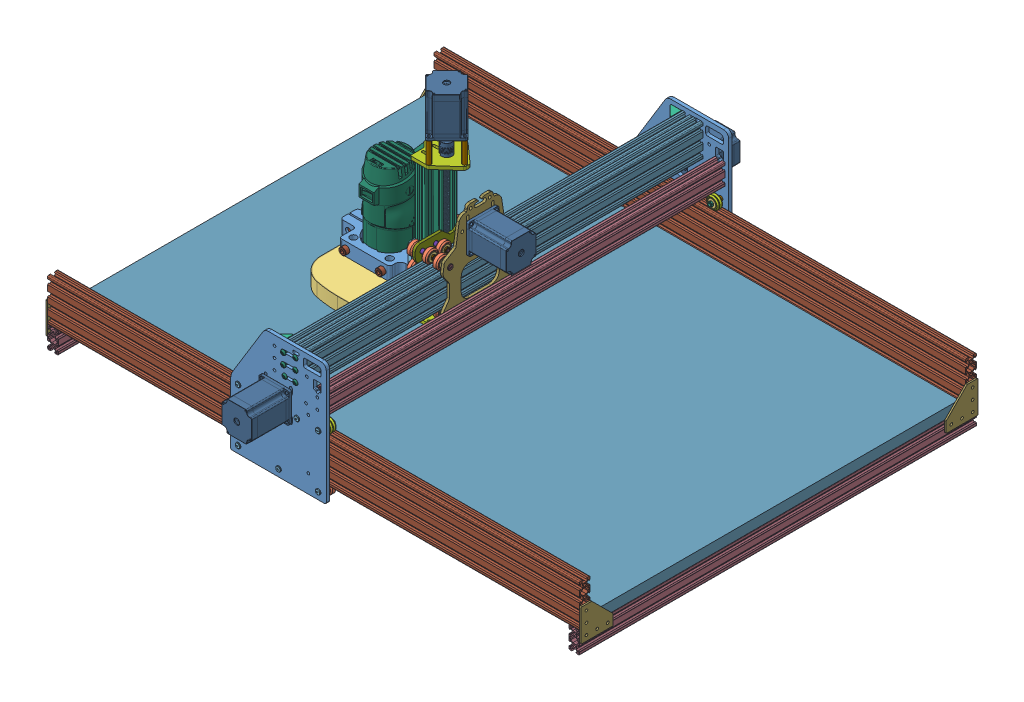
SolidWorks assembly MainFrame, configuration Default. Lengths in mm.
Overall size (1006.09 487.54 917.5).
449 component instances, 49 part files, 68 mates.
Components (placement in the parent):
- LeftSideGantry-1: LeftSideGantry [Default] at (4.6712 -16.6579 18.9022) size (180.04 227.49 106.2)
  - Gantry-SidePlate-1: Gantry-SidePlate [Default] at (69.6077 16.1075 4.3758) size (180.04 227.49 6.35)
  - SolidWheelWithEccentric-1: SolidWheelWithEccentric [Default] at (93.8735 -103.2758 -22.2954) size (23.89 23.89 29.6)
    - Delrin Solid V-Wheel-1: Delrin Solid V-Wheel [Default] at (-54.4571 19.9667 15.1712) size (23.89 23.89 10.23)
    - Precision Ball Bearing-1: Precision Ball Bearing [Default] at (-54.4571 19.9667 12.1712) x (0 0 1) z (-1 0 0) size (5 16 16)
    - Precision Ball Bearing-2: Precision Ball Bearing [Default] at (-54.4571 19.9667 18.1712) x (0 0 -1) z (1 0 0) size (5 16 16)
    - Steel Eccentric Spacer-1: Steel Eccentric Spacer [Default] at (-55.2471 19.9667 26.6712) x (0 0 -1) z (1 0 0) size (7.27 9.09 7.9)
    - 5mm Low Profile Socket Head Screw - Multiple Lengths-1: 5mm Low Profile Socket Head Screw - Multiple Lengths [Default] at (-54.4571 19.9667 34.7712) x (0 0 -1) z (1 0 0) size (27.2 9.5 9.5)
    - Nylon Insert Hex Locknut 5mm-1: Nylon Insert Hex Locknut 5mm [Default] at (-54.4571 19.9667 9.6712) x (-0.923728 -0.383049 0) z (0 0 -1) size (7.68 8.82 4.5)
  - SolidWheelWithEccentric-2: SolidWheelWithEccentric [Default] at (19.3435 -103.2758 -22.2954) size (23.89 23.89 29.6)
    - Delrin Solid V-Wheel-1: Delrin Solid V-Wheel [Default] at (-54.4571 19.9667 15.1712) size (23.89 23.89 10.23)
    - Precision Ball Bearing-1: Precision Ball Bearing [Default] at (-54.4571 19.9667 12.1712) x (0 0 1) z (-1 0 0) size (5 16 16)
    - Precision Ball Bearing-2: Precision Ball Bearing [Default] at (-54.4571 19.9667 18.1712) x (0 0 -1) z (1 0 0) size (5 16 16)
    - Steel Eccentric Spacer-1: Steel Eccentric Spacer [Default] at (-55.2471 19.9667 26.6712) x (0 0 -1) z (1 0 0) size (7.27 9.09 7.9)
    - 5mm Low Profile Socket Head Screw - Multiple Lengths-1: 5mm Low Profile Socket Head Screw - Multiple Lengths [Default] at (-54.4571 19.9667 34.7712) x (0 0 -1) z (1 0 0) size (27.2 9.5 9.5)
    - Nylon Insert Hex Locknut 5mm-1: Nylon Insert Hex Locknut 5mm [Default] at (-54.4571 19.9667 9.6712) x (-0.923728 -0.383049 0) z (0 0 -1) size (7.68 8.82 4.5)
  - SolidWheelWithEccentric-3: SolidWheelWithEccentric [Default] at (-56.7665 -103.2758 -22.2954) size (23.89 23.89 29.6)
    - Delrin Solid V-Wheel-1: Delrin Solid V-Wheel [Default] at (-54.4571 19.9667 15.1712) size (23.89 23.89 10.23)
    - Precision Ball Bearing-1: Precision Ball Bearing [Default] at (-54.4571 19.9667 12.1712) x (0 0 1) z (-1 0 0) size (5 16 16)
    - Precision Ball Bearing-2: Precision Ball Bearing [Default] at (-54.4571 19.9667 18.1712) x (0 0 -1) z (1 0 0) size (5 16 16)
    - Steel Eccentric Spacer-1: Steel Eccentric Spacer [Default] at (-55.2471 19.9667 26.6712) x (0 0 -1) z (1 0 0) size (7.27 9.09 7.9)
    - 5mm Low Profile Socket Head Screw - Multiple Lengths-1: 5mm Low Profile Socket Head Screw - Multiple Lengths [Default] at (-54.4571 19.9667 34.7712) x (0 0 -1) z (1 0 0) size (27.2 9.5 9.5)
    - Nylon Insert Hex Locknut 5mm-1: Nylon Insert Hex Locknut 5mm [Default] at (-54.4571 19.9667 9.6712) x (-0.923728 -0.383049 0) z (0 0 -1) size (7.68 8.82 4.5)
  - V-Slot Delrin Dual Wheel Assembly-1: V-Slot Delrin Dual Wheel Assembly [Default] at (-115.4002 2.9807 3.6104) size (23.89 23.89 29.95)
    - Delrin Dual V-Wheel-1: Delrin Dual V-Wheel [Default] at (4.1766 13.0717 -11.0846) size (23.89 23.89 10.23)
    - Precision Ball Bearing-1: Precision Ball Bearing [Default] at (4.1766 13.0717 -8.0846) x (0 0 -1) z (1 0 0) size (5 16 16)
    - Precision Ball Bearing-2: Precision Ball Bearing [Default] at (4.1766 13.0717 -14.0846) x (0 0 -1) z (1 0 0) size (5 16 16)
    - 5mm Precision Washer-1: 5mm Precision Washer [Default] at (4.1766 13.0717 -11.5846) x (0 0 1) z (-1 0 0) size (1 10 10)
    - .25 Inch Aluminum Spacer-1: .25 Inch Aluminum Spacer [Default] at (4.1766 13.0717 0.7654) x (0 0 -1) z (1 0 0) size (6.35 8 8)
    - 5mm Low Profile Socket Head Screw - Multiple Lengths-1: 5mm Low Profile Socket Head Screw - Multiple Lengths [Default] at (4.1766 13.0717 8.8654) x (0 0 -1) z (1 0 0) size (27.2 9.5 9.5)
    - Nylon Insert Hex Locknut 5mm-1: Nylon Insert Hex Locknut 5mm [Default] at (4.1766 13.0717 -16.5846) x (-0.923728 -0.383049 0) z (0 0 -1) size (7.68 8.82 4.5)
  - V-Slot Delrin Dual Wheel Assembly-2: V-Slot Delrin Dual Wheel Assembly [Default] at (-75.4002 2.9807 3.6104) size (23.89 23.89 29.95)
    - Delrin Dual V-Wheel-1: Delrin Dual V-Wheel [Default] at (4.1766 13.0717 -11.0846) size (23.89 23.89 10.23)
    - Precision Ball Bearing-1: Precision Ball Bearing [Default] at (4.1766 13.0717 -8.0846) x (0 0 -1) z (1 0 0) size (5 16 16)
    - Precision Ball Bearing-2: Precision Ball Bearing [Default] at (4.1766 13.0717 -14.0846) x (0 0 -1) z (1 0 0) size (5 16 16)
    - 5mm Precision Washer-1: 5mm Precision Washer [Default] at (4.1766 13.0717 -11.5846) x (0 0 1) z (-1 0 0) size (1 10 10)
    - .25 Inch Aluminum Spacer-1: .25 Inch Aluminum Spacer [Default] at (4.1766 13.0717 0.7654) x (0 0 -1) z (1 0 0) size (6.35 8 8)
    - 5mm Low Profile Socket Head Screw - Multiple Lengths-1: 5mm Low Profile Socket Head Screw - Multiple Lengths [Default] at (4.1766 13.0717 8.8654) x (0 0 -1) z (1 0 0) size (27.2 9.5 9.5)
    - Nylon Insert Hex Locknut 5mm-1: Nylon Insert Hex Locknut 5mm [Default] at (4.1766 13.0717 -16.5846) x (-0.923728 -0.383049 0) z (0 0 -1) size (7.68 8.82 4.5)
  - V-Slot Delrin Dual Wheel Assembly-3: V-Slot Delrin Dual Wheel Assembly [Default] at (35.1946 3.1996 3.6104) size (23.89 23.89 29.95)
    - Delrin Dual V-Wheel-1: Delrin Dual V-Wheel [Default] at (4.1766 13.0717 -11.0846) size (23.89 23.89 10.23)
    - Precision Ball Bearing-1: Precision Ball Bearing [Default] at (4.1766 13.0717 -8.0846) x (0 0 -1) z (1 0 0) size (5 16 16)
    - Precision Ball Bearing-2: Precision Ball Bearing [Default] at (4.1766 13.0717 -14.0846) x (0 0 -1) z (1 0 0) size (5 16 16)
    - 5mm Precision Washer-1: 5mm Precision Washer [Default] at (4.1766 13.0717 -11.5846) x (0 0 1) z (-1 0 0) size (1 10 10)
    - .25 Inch Aluminum Spacer-1: .25 Inch Aluminum Spacer [Default] at (4.1766 13.0717 0.7654) x (0 0 -1) z (1 0 0) size (6.35 8 8)
    - 5mm Low Profile Socket Head Screw - Multiple Lengths-1: 5mm Low Profile Socket Head Screw - Multiple Lengths [Default] at (4.1766 13.0717 8.8654) x (0 0 -1) z (1 0 0) size (27.2 9.5 9.5)
    - Nylon Insert Hex Locknut 5mm-1: Nylon Insert Hex Locknut 5mm [Default] at (4.1766 13.0717 -16.5846) x (-0.923728 -0.383049 0) z (0 0 -1) size (7.68 8.82 4.5)
  - V-Slot Delrin Dual Wheel Assembly-4: V-Slot Delrin Dual Wheel Assembly [Default] at (-4.7602 2.9807 3.6104) size (23.89 23.89 29.95)
    - Delrin Dual V-Wheel-1: Delrin Dual V-Wheel [Default] at (4.1766 13.0717 -11.0846) size (23.89 23.89 10.23)
    - Precision Ball Bearing-1: Precision Ball Bearing [Default] at (4.1766 13.0717 -8.0846) x (0 0 -1) z (1 0 0) size (5 16 16)
    - Precision Ball Bearing-2: Precision Ball Bearing [Default] at (4.1766 13.0717 -14.0846) x (0 0 -1) z (1 0 0) size (5 16 16)
    - 5mm Precision Washer-1: 5mm Precision Washer [Default] at (4.1766 13.0717 -11.5846) x (0 0 1) z (-1 0 0) size (1 10 10)
    - .25 Inch Aluminum Spacer-1: .25 Inch Aluminum Spacer [Default] at (4.1766 13.0717 0.7654) x (0 0 -1) z (1 0 0) size (6.35 8 8)
    - 5mm Low Profile Socket Head Screw - Multiple Lengths-1: 5mm Low Profile Socket Head Screw - Multiple Lengths [Default] at (4.1766 13.0717 8.8654) x (0 0 -1) z (1 0 0) size (27.2 9.5 9.5)
    - Nylon Insert Hex Locknut 5mm-1: Nylon Insert Hex Locknut 5mm [Default] at (4.1766 13.0717 -16.5846) x (-0.923728 -0.383049 0) z (0 0 -1) size (7.68 8.82 4.5)
  - stepper motor NEMA 23 57x76-1: stepper motor NEMA 23 57x76 [По умолчанию] at (-36.1116 31.8353 88.7258) x (0.999999 0.00168 0) z (-0.00168 0.999999 0) size (56.67 96.5 56.58)
- vslot_20_x_80-1: vslot_20_x_80 [Default] at (526.5598 -49.8299 11.278) x (0.001454 -0.999999 0) z (-0.999999 -0.001454 0) size (80 20 1000)
- RightSideGantry-1: RightSideGantry [Default] at (45.1481 -36.7387 -745.9581) size (182.59 229.13 105)
  - Gantry-SidePlate-1: Gantry-SidePlate [Default] at (29.1308 36.1882 12.8861) size (180.04 227.49 6.35)
  - V-Slot Delrin Dual Wheel Assembly-1: V-Slot Delrin Dual Wheel Assembly [Default] at (-120.5656 46.608 20.0014) x (0.923728 0.383049 0) z (0 0 -1) size (23.89 23.89 29.95)
    - Delrin Dual V-Wheel-1: Delrin Dual V-Wheel [Default] at (4.1766 13.0717 -11.0846) size (23.89 23.89 10.23)
    - Precision Ball Bearing-1: Precision Ball Bearing [Default] at (4.1766 13.0717 -8.0846) x (0 0 -1) z (1 0 0) size (5 16 16)
    - Precision Ball Bearing-2: Precision Ball Bearing [Default] at (4.1766 13.0717 -14.0846) x (0 0 -1) z (1 0 0) size (5 16 16)
    - 5mm Precision Washer-1: 5mm Precision Washer [Default] at (4.1766 13.0717 -11.5846) x (0 0 1) z (-1 0 0) size (1 10 10)
    - .25 Inch Aluminum Spacer-1: .25 Inch Aluminum Spacer [Default] at (4.1766 13.0717 0.7654) x (0 0 -1) z (1 0 0) size (6.35 8 8)
    - 5mm Low Profile Socket Head Screw - Multiple Lengths-1: 5mm Low Profile Socket Head Screw - Multiple Lengths [Default] at (4.1766 13.0717 8.8654) x (0 0 -1) z (1 0 0) size (27.2 9.5 9.5)
    - Nylon Insert Hex Locknut 5mm-1: Nylon Insert Hex Locknut 5mm [Default] at (4.1766 13.0717 -16.5846) x (-0.923728 -0.383049 0) z (0 0 -1) size (7.68 8.82 4.5)
  - V-Slot Delrin Dual Wheel Assembly-2: V-Slot Delrin Dual Wheel Assembly [Default] at (-160.5656 46.608 20.0014) x (0.923728 0.383049 0) z (0 0 -1) size (23.89 23.89 29.95)
    - Delrin Dual V-Wheel-1: Delrin Dual V-Wheel [Default] at (4.1766 13.0717 -11.0846) size (23.89 23.89 10.23)
    - Precision Ball Bearing-1: Precision Ball Bearing [Default] at (4.1766 13.0717 -8.0846) x (0 0 -1) z (1 0 0) size (5 16 16)
    - Precision Ball Bearing-2: Precision Ball Bearing [Default] at (4.1766 13.0717 -14.0846) x (0 0 -1) z (1 0 0) size (5 16 16)
    - 5mm Precision Washer-1: 5mm Precision Washer [Default] at (4.1766 13.0717 -11.5846) x (0 0 1) z (-1 0 0) size (1 10 10)
    - .25 Inch Aluminum Spacer-1: .25 Inch Aluminum Spacer [Default] at (4.1766 13.0717 0.7654) x (0 0 -1) z (1 0 0) size (6.35 8 8)
    - 5mm Low Profile Socket Head Screw - Multiple Lengths-1: 5mm Low Profile Socket Head Screw - Multiple Lengths [Default] at (4.1766 13.0717 8.8654) x (0 0 -1) z (1 0 0) size (27.2 9.5 9.5)
    - Nylon Insert Hex Locknut 5mm-1: Nylon Insert Hex Locknut 5mm [Default] at (4.1766 13.0717 -16.5846) x (-0.923728 -0.383049 0) z (0 0 -1) size (7.68 8.82 4.5)
  - V-Slot Delrin Dual Wheel Assembly-3: V-Slot Delrin Dual Wheel Assembly [Default] at (7.7594 25.8772 20.0014) x (-0.923728 -0.383049 0) z (0 0 -1) size (23.89 23.89 29.95)
    - Delrin Dual V-Wheel-1: Delrin Dual V-Wheel [Default] at (4.1766 13.0717 -11.0846) size (23.89 23.89 10.23)
    - Precision Ball Bearing-1: Precision Ball Bearing [Default] at (4.1766 13.0717 -8.0846) x (0 0 -1) z (1 0 0) size (5 16 16)
    - Precision Ball Bearing-2: Precision Ball Bearing [Default] at (4.1766 13.0717 -14.0846) x (0 0 -1) z (1 0 0) size (5 16 16)
    - 5mm Precision Washer-1: 5mm Precision Washer [Default] at (4.1766 13.0717 -11.5846) x (0 0 1) z (-1 0 0) size (1 10 10)
    - .25 Inch Aluminum Spacer-1: .25 Inch Aluminum Spacer [Default] at (4.1766 13.0717 0.7654) x (0 0 -1) z (1 0 0) size (6.35 8 8)
    - 5mm Low Profile Socket Head Screw - Multiple Lengths-1: 5mm Low Profile Socket Head Screw - Multiple Lengths [Default] at (4.1766 13.0717 8.8654) x (0 0 -1) z (1 0 0) size (27.2 9.5 9.5)
    - Nylon Insert Hex Locknut 5mm-1: Nylon Insert Hex Locknut 5mm [Default] at (4.1766 13.0717 -16.5846) x (-0.923728 -0.383049 0) z (0 0 -1) size (7.68 8.82 4.5)
  - V-Slot Delrin Dual Wheel Assembly-4: V-Slot Delrin Dual Wheel Assembly [Default] at (-32.1954 25.6582 20.0014) x (-0.923728 -0.383049 0) z (0 0 -1) size (23.89 23.89 29.95)
    - Delrin Dual V-Wheel-1: Delrin Dual V-Wheel [Default] at (4.1766 13.0717 -11.0846) size (23.89 23.89 10.23)
    - Precision Ball Bearing-1: Precision Ball Bearing [Default] at (4.1766 13.0717 -8.0846) x (0 0 -1) z (1 0 0) size (5 16 16)
    - Precision Ball Bearing-2: Precision Ball Bearing [Default] at (4.1766 13.0717 -14.0846) x (0 0 -1) z (1 0 0) size (5 16 16)
    - 5mm Precision Washer-1: 5mm Precision Washer [Default] at (4.1766 13.0717 -11.5846) x (0 0 1) z (-1 0 0) size (1 10 10)
    - .25 Inch Aluminum Spacer-1: .25 Inch Aluminum Spacer [Default] at (4.1766 13.0717 0.7654) x (0 0 -1) z (1 0 0) size (6.35 8 8)
    - 5mm Low Profile Socket Head Screw - Multiple Lengths-1: 5mm Low Profile Socket Head Screw - Multiple Lengths [Default] at (4.1766 13.0717 8.8654) x (0 0 -1) z (1 0 0) size (27.2 9.5 9.5)
    - Nylon Insert Hex Locknut 5mm-1: Nylon Insert Hex Locknut 5mm [Default] at (4.1766 13.0717 -16.5846) x (-0.923728 -0.383049 0) z (0 0 -1) size (7.68 8.82 4.5)
  - SolidWheelWithEccentric-1: SolidWheelWithEccentric [Default] at (-108.3154 -23.6223 45.9073) x (0.923728 0.383049 0) z (0 0 -1) size (23.89 23.89 29.6)
    - Delrin Solid V-Wheel-1: Delrin Solid V-Wheel [Default] at (-54.4571 19.9667 15.1712) size (23.89 23.89 10.23)
    - Precision Ball Bearing-1: Precision Ball Bearing [Default] at (-54.4571 19.9667 12.1712) x (0 0 1) z (-1 0 0) size (5 16 16)
    - Precision Ball Bearing-2: Precision Ball Bearing [Default] at (-54.4571 19.9667 18.1712) x (0 0 -1) z (1 0 0) size (5 16 16)
    - Steel Eccentric Spacer-1: Steel Eccentric Spacer [Default] at (-55.2471 19.9667 26.6712) x (0 0 -1) z (1 0 0) size (7.27 9.09 7.9)
    - 5mm Low Profile Socket Head Screw - Multiple Lengths-1: 5mm Low Profile Socket Head Screw - Multiple Lengths [Default] at (-54.4571 19.9667 34.7712) x (0 0 -1) z (1 0 0) size (27.2 9.5 9.5)
    - Nylon Insert Hex Locknut 5mm-1: Nylon Insert Hex Locknut 5mm [Default] at (-54.4571 19.9667 9.6712) x (-0.923728 -0.383049 0) z (0 0 -1) size (7.68 8.82 4.5)
  - SolidWheelWithEccentric-2: SolidWheelWithEccentric [Default] at (-32.9954 -23.6223 45.9073) x (0.923728 0.383049 0) z (0 0 -1) size (23.89 23.89 29.6)
    - Delrin Solid V-Wheel-1: Delrin Solid V-Wheel [Default] at (-54.4571 19.9667 15.1712) size (23.89 23.89 10.23)
    - Precision Ball Bearing-1: Precision Ball Bearing [Default] at (-54.4571 19.9667 12.1712) x (0 0 1) z (-1 0 0) size (5 16 16)
    - Precision Ball Bearing-2: Precision Ball Bearing [Default] at (-54.4571 19.9667 18.1712) x (0 0 -1) z (1 0 0) size (5 16 16)
    - Steel Eccentric Spacer-1: Steel Eccentric Spacer [Default] at (-55.2471 19.9667 26.6712) x (0 0 -1) z (1 0 0) size (7.27 9.09 7.9)
    - 5mm Low Profile Socket Head Screw - Multiple Lengths-1: 5mm Low Profile Socket Head Screw - Multiple Lengths [Default] at (-54.4571 19.9667 34.7712) x (0 0 -1) z (1 0 0) size (27.2 9.5 9.5)
    - Nylon Insert Hex Locknut 5mm-1: Nylon Insert Hex Locknut 5mm [Default] at (-54.4571 19.9667 9.6712) x (-0.923728 -0.383049 0) z (0 0 -1) size (7.68 8.82 4.5)
  - SolidWheelWithEccentric-3: SolidWheelWithEccentric [Default] at (42.3246 -23.6223 45.9073) x (0.923728 0.383049 0) z (0 0 -1) size (23.89 23.89 29.6)
    - Delrin Solid V-Wheel-1: Delrin Solid V-Wheel [Default] at (-54.4571 19.9667 15.1712) size (23.89 23.89 10.23)
    - Precision Ball Bearing-1: Precision Ball Bearing [Default] at (-54.4571 19.9667 12.1712) x (0 0 1) z (-1 0 0) size (5 16 16)
    - Precision Ball Bearing-2: Precision Ball Bearing [Default] at (-54.4571 19.9667 18.1712) x (0 0 -1) z (1 0 0) size (5 16 16)
    - Steel Eccentric Spacer-1: Steel Eccentric Spacer [Default] at (-55.2471 19.9667 26.6712) x (0 0 -1) z (1 0 0) size (7.27 9.09 7.9)
    - 5mm Low Profile Socket Head Screw - Multiple Lengths-1: 5mm Low Profile Socket Head Screw - Multiple Lengths [Default] at (-54.4571 19.9667 34.7712) x (0 0 -1) z (1 0 0) size (27.2 9.5 9.5)
    - Nylon Insert Hex Locknut 5mm-1: Nylon Insert Hex Locknut 5mm [Default] at (-54.4571 19.9667 9.6712) x (-0.923728 -0.383049 0) z (0 0 -1) size (7.68 8.82 4.5)
  - stepper motor NEMA 23 57x76-1: stepper motor NEMA 23 57x76 [По умолчанию] at (-76.1724 47.1139 -63.9139) x (1 0 0) z (0 -1 0) size (56.67 96.5 56.58)
- vslot_20_x_80-2: vslot_20_x_80 [Default] at (526.5598 -49.8299 -714.722) x (0.001454 -0.999999 0) z (-0.999999 -0.001454 0) size (80 20 1000)
- CrossSlideAssembly-1: CrossSlideAssembly [Default] at (27.0126 95.3807 -262.4793) x (0 0 1) z (-1 0 0) size (140.04 177.38 107.28)
  - Gantry-Mount-1: Gantry-Mount [Default] at (-125.7398 -49.8559 3.7822) size (140.04 177.38 9.53)
  - Steel Eccentric Spacer-1: Steel Eccentric Spacer [Default] at (-94.6645 20.3573 14.5772) x (0 0 1) z (-0.00681 0.999977 0) size (7.27 9.09 7.9)
  - Steel Eccentric Spacer-2: Steel Eccentric Spacer [Default] at (19.1018 20.3573 14.5772) x (0 0 1) z (-0.00681 0.999977 0) size (7.27 9.09 7.9)
  - .25 Inch Aluminum Spacer-3: .25 Inch Aluminum Spacer [Default] at (19.1049 -57.7227 19.6572) x (0 0 -1) z (1 0 0) size (6.35 8 8)
  - .25 Inch Aluminum Spacer-4: .25 Inch Aluminum Spacer [Default] at (-94.6784 -57.7227 19.6572) x (0 0 -1) z (1 0 0) size (6.35 8 8)
  - SolidWheel-7: SolidWheel [Default] at (56.5607 -62.4006 9.4904) size (23.89 23.89 11)
    - Delrin Solid V-Wheel-1: Delrin Solid V-Wheel [Default] at (-37.4558 4.6779 16.5868) size (23.89 23.89 10.23)
    - Precision Ball Bearing-1: Precision Ball Bearing [Default] at (-37.4558 4.6779 19.5868) x (0 0 -1) z (1 0 0) size (5 16 16)
    - Precision Ball Bearing-2: Precision Ball Bearing [Default] at (-37.4558 4.6779 13.5868) x (0 0 1) z (-1 0 0) size (5 16 16)
  - SolidWheel-8: SolidWheel [Default] at (56.5522 16.4694 9.4904) size (23.89 23.89 11)
    - Delrin Solid V-Wheel-1: Delrin Solid V-Wheel [Default] at (-37.4558 4.6779 16.5868) size (23.89 23.89 10.23)
    - Precision Ball Bearing-1: Precision Ball Bearing [Default] at (-37.4558 4.6779 19.5868) x (0 0 -1) z (1 0 0) size (5 16 16)
    - Precision Ball Bearing-2: Precision Ball Bearing [Default] at (-37.4558 4.6779 13.5868) x (0 0 1) z (-1 0 0) size (5 16 16)
  - SolidWheel-9: SolidWheel [Default] at (-57.2141 16.4694 9.4904) size (23.89 23.89 11)
    - Delrin Solid V-Wheel-1: Delrin Solid V-Wheel [Default] at (-37.4558 4.6779 16.5868) size (23.89 23.89 10.23)
    - Precision Ball Bearing-1: Precision Ball Bearing [Default] at (-37.4558 4.6779 19.5868) x (0 0 -1) z (1 0 0) size (5 16 16)
    - Precision Ball Bearing-2: Precision Ball Bearing [Default] at (-37.4558 4.6779 13.5868) x (0 0 1) z (-1 0 0) size (5 16 16)
  - SolidWheel-10: SolidWheel [Default] at (-57.2226 -62.4006 9.4904) size (23.89 23.89 11)
    - Delrin Solid V-Wheel-1: Delrin Solid V-Wheel [Default] at (-37.4558 4.6779 16.5868) size (23.89 23.89 10.23)
    - Precision Ball Bearing-1: Precision Ball Bearing [Default] at (-37.4558 4.6779 19.5868) x (0 0 -1) z (1 0 0) size (5 16 16)
    - Precision Ball Bearing-2: Precision Ball Bearing [Default] at (-37.4558 4.6779 13.5868) x (0 0 1) z (-1 0 0) size (5 16 16)
  - Low Profile Socket Head Screw-2: Low Profile Socket Head Screw [Default] at (19.0964 21.1473 6.7947) x (0 0 1) z (-0.923728 -0.383049 0) size (32.23 9.5 9.5)
  - Low Profile Socket Head Screw-3: Low Profile Socket Head Screw [Default] at (-94.6699 21.1473 6.7947) x (0 0 1) z (-0.923728 -0.383049 0) size (32.23 9.5 9.5)
  - Low Profile Socket Head Screw-11: Low Profile Socket Head Screw [Default] at (19.1049 -57.7227 6.7947) x (0 0 1) z (-0.923728 -0.383049 0) size (32.23 9.5 9.5)
  - Low Profile Socket Head Screw-12: Low Profile Socket Head Screw [Default] at (-94.6784 -57.7227 6.7947) x (0 0 1) z (-0.923728 -0.383049 0) size (32.23 9.5 9.5)
  - stepper motor NEMA 23 57x76-1: stepper motor NEMA 23 57x76 [По умолчанию] at (-37.9748 53.7319 -68.2553) x (1 0 0) z (0 -1 0) size (56.67 96.5 56.58)
- vslot 20 x 60-1: vslot 20 x 60 [Default] at (6.4261 6.4154 -443.5992) x (0 -1 0) z (0 0 -1) size (60 20 770.25)
  - vslot_20_x_60-1: vslot_20_x_60 [Default] at (-59.9677 5.5907 273.1228) size (60 20 750)
  - socket button head cap screw_am-1: socket button head cap screw_am [B18.3.4M - 5 x 0.8 x 16 SBHCS --N] at (-49.9677 5.5907 291.8728) x (0 0 -1) z (1 0 0) size (18.75 9.5 9.5)
  - socket button head cap screw_am-2: socket button head cap screw_am [B18.3.4M - 5 x 0.8 x 16 SBHCS --N] at (-69.9677 5.5907 294.6228) x (0 0 -1) z (1 0 0) size (18.75 9.5 9.5)
  - socket button head cap screw_am-3: socket button head cap screw_am [B18.3.4M - 5 x 0.8 x 16 SBHCS --N] at (-89.9677 5.5907 294.6228) x (0 0 -1) z (1 0 0) size (18.75 9.5 9.5)
  - socket button head cap screw_am-4: socket button head cap screw_am [B18.3.4M - 5 x 0.8 x 16 SBHCS --N] at (-89.9677 5.5907 -475.6272) x (0 0 1) z (-1 0 0) size (18.75 9.5 9.5)
  - socket button head cap screw_am-5: socket button head cap screw_am [B18.3.4M - 5 x 0.8 x 16 SBHCS --N] at (-69.9677 5.5907 -475.6272) x (0 0 1) z (-1 0 0) size (18.75 9.5 9.5)
  - socket button head cap screw_am-6: socket button head cap screw_am [B18.3.4M - 5 x 0.8 x 16 SBHCS --N] at (-49.9677 5.5907 -475.6272) x (0 0 1) z (0.888663 -0.45856 0) size (18.75 9.5 9.5)
- vslot 20 x 60-2: vslot 20 x 60 [Default] at (-24.7553 6.4154 -259.8448) x (0 -1 0) z (0 0 1) size (60 20 770.25)
  - vslot_20_x_60-1: vslot_20_x_60 [Default] at (-59.9677 5.5907 273.1228) size (60 20 750)
  - socket button head cap screw_am-1: socket button head cap screw_am [B18.3.4M - 5 x 0.8 x 16 SBHCS --N] at (-49.9677 5.5907 291.8728) x (0 0 -1) z (1 0 0) size (18.75 9.5 9.5)
  - socket button head cap screw_am-2: socket button head cap screw_am [B18.3.4M - 5 x 0.8 x 16 SBHCS --N] at (-69.9677 5.5907 294.6228) x (0 0 -1) z (1 0 0) size (18.75 9.5 9.5)
  - socket button head cap screw_am-3: socket button head cap screw_am [B18.3.4M - 5 x 0.8 x 16 SBHCS --N] at (-89.9677 5.5907 294.6228) x (0 0 -1) z (1 0 0) size (18.75 9.5 9.5)
  - socket button head cap screw_am-4: socket button head cap screw_am [B18.3.4M - 5 x 0.8 x 16 SBHCS --N] at (-89.9677 5.5907 -475.6272) x (0 0 1) z (-1 0 0) size (18.75 9.5 9.5)
  - socket button head cap screw_am-5: socket button head cap screw_am [B18.3.4M - 5 x 0.8 x 16 SBHCS --N] at (-69.9677 5.5907 -475.6272) x (0 0 1) z (-1 0 0) size (18.75 9.5 9.5)
  - socket button head cap screw_am-6: socket button head cap screw_am [B18.3.4M - 5 x 0.8 x 16 SBHCS --N] at (-49.9677 5.5907 -475.6272) x (0 0 1) z (0.888663 -0.45856 0) size (18.75 9.5 9.5)
- FrontGantryPlateZaxis-1: FrontGantryPlateZaxis [Default] at (-15.5555 68.0354 -249.6907) x (0 0 1) z (-1 0 0) size (140.04 377.73 80.67)
  - Gantry-Mount-Part2-1: Gantry-Mount-Part2 [Default] at (-50.6115 110.7452 18.3591) size (140.04 106.72 4.76)
  - SolidWheelWithSpacer-4: SolidWheelWithSpacer [Default] at (-86.321 51.345 -9.6249) size (23.89 23.89 32.23)
    - SolidWheel-1: SolidWheel [Default] at (16.2383 -7.5303 -3.4528) size (23.89 23.89 11)
      - Delrin Solid V-Wheel-1: Delrin Solid V-Wheel [Default] at (-37.4558 4.6779 16.5868) size (23.89 23.89 10.23)
      - Precision Ball Bearing-1: Precision Ball Bearing [Default] at (-37.4558 4.6779 19.5868) x (0 0 -1) z (1 0 0) size (5 16 16)
      - Precision Ball Bearing-2: Precision Ball Bearing [Default] at (-37.4558 4.6779 13.5868) x (0 0 1) z (-1 0 0) size (5 16 16)
    - Low Profile Socket Head Screw-1: Low Profile Socket Head Screw [Default] at (-21.2174 -2.8524 35.734) x (0 0 -1) z (-0.923728 -0.383049 0) size (32.23 9.5 9.5)
    - .25 Inch Nylon Spacer-1: .25 Inch Nylon Spacer [Default] at (-21.2174 -2.8524 27.984) x (0 0 -1) z (1 0 0) size (6.35 7.94 7.94)
    - hex nut jam_am-1: hex nut jam_am [B18.2.4.5M - Hex jam nut,  M5 x 0.8 --D-N] at (-21.2174 -2.8524 7.634) size (8 9.24 2.7)
    - 3mm Aluminum Spacer-1: 3mm Aluminum Spacer [Default] at (-21.2174 -2.8524 21.634) x (0 0 -1) z (1 0 0) size (3 8 8)
  - SolidWheelWithSpacer-5: SolidWheelWithSpacer [Default] at (27.5253 51.345 -9.6249) size (23.89 23.89 32.23)
    - SolidWheel-1: SolidWheel [Default] at (16.2383 -7.5303 -3.4528) size (23.89 23.89 11)
      - Delrin Solid V-Wheel-1: Delrin Solid V-Wheel [Default] at (-37.4558 4.6779 16.5868) size (23.89 23.89 10.23)
      - Precision Ball Bearing-1: Precision Ball Bearing [Default] at (-37.4558 4.6779 19.5868) x (0 0 -1) z (1 0 0) size (5 16 16)
      - Precision Ball Bearing-2: Precision Ball Bearing [Default] at (-37.4558 4.6779 13.5868) x (0 0 1) z (-1 0 0) size (5 16 16)
    - Low Profile Socket Head Screw-1: Low Profile Socket Head Screw [Default] at (-21.2174 -2.8524 35.734) x (0 0 -1) z (-0.923728 -0.383049 0) size (32.23 9.5 9.5)
    - .25 Inch Nylon Spacer-1: .25 Inch Nylon Spacer [Default] at (-21.2174 -2.8524 27.984) x (0 0 -1) z (1 0 0) size (6.35 7.94 7.94)
    - hex nut jam_am-1: hex nut jam_am [B18.2.4.5M - Hex jam nut,  M5 x 0.8 --D-N] at (-21.2174 -2.8524 7.634) size (8 9.24 2.7)
    - 3mm Aluminum Spacer-1: 3mm Aluminum Spacer [Default] at (-21.2174 -2.8524 21.634) x (0 0 -1) z (1 0 0) size (3 8 8)
  - SolidWheelWithEccentric2-4: SolidWheelWithEccentric2 [Default] at (-75.4106 -21.8202 -18.8913) size (23.89 23.89 32.23)
    - SolidWheel-1: SolidWheel [Default] at (5.3595 -13.235 6.1636) size (23.89 23.89 11)
      - Delrin Solid V-Wheel-1: Delrin Solid V-Wheel [Default] at (-37.4558 4.6779 16.5868) size (23.89 23.89 10.23)
      - Precision Ball Bearing-1: Precision Ball Bearing [Default] at (-37.4558 4.6779 19.5868) x (0 0 -1) z (1 0 0) size (5 16 16)
      - Precision Ball Bearing-2: Precision Ball Bearing [Default] at (-37.4558 4.6779 13.5868) x (0 0 1) z (-1 0 0) size (5 16 16)
    - Steel Eccentric Spacer-1: Steel Eccentric Spacer [Default] at (-32.1017 -9.3471 37.2504) x (0 0 -1) z (0.00681 0.999977 0) size (7.27 9.09 7.9)
    - Low Profile Socket Head Screw-1: Low Profile Socket Head Screw [Default] at (-32.0963 -8.5571 45.0004) x (0 0 -1) z (1 0 0) size (32.23 9.5 9.5)
    - hex nut jam_am-1: hex nut jam_am [B18.2.4.5M - Hex jam nut,  M5 x 0.8 --D-N] at (-32.0963 -8.5571 17.2504) size (8 9.24 2.7)
    - 3mm Aluminum Spacer-1: 3mm Aluminum Spacer [Default] at (-32.0963 -8.5571 31.2504) x (0 0 -1) z (1 0 0) size (3 8 8)
  - SolidWheelWithEccentric2-5: SolidWheelWithEccentric2 [Default] at (38.3727 -21.8202 -18.8913) size (23.89 23.89 32.23)
    - SolidWheel-1: SolidWheel [Default] at (5.3595 -13.235 6.1636) size (23.89 23.89 11)
      - Delrin Solid V-Wheel-1: Delrin Solid V-Wheel [Default] at (-37.4558 4.6779 16.5868) size (23.89 23.89 10.23)
      - Precision Ball Bearing-1: Precision Ball Bearing [Default] at (-37.4558 4.6779 19.5868) x (0 0 -1) z (1 0 0) size (5 16 16)
      - Precision Ball Bearing-2: Precision Ball Bearing [Default] at (-37.4558 4.6779 13.5868) x (0 0 1) z (-1 0 0) size (5 16 16)
    - Steel Eccentric Spacer-1: Steel Eccentric Spacer [Default] at (-32.1017 -9.3471 37.2504) x (0 0 -1) z (0.00681 0.999977 0) size (7.27 9.09 7.9)
    - Low Profile Socket Head Screw-1: Low Profile Socket Head Screw [Default] at (-32.0963 -8.5571 45.0004) x (0 0 -1) z (1 0 0) size (32.23 9.5 9.5)
    - hex nut jam_am-1: hex nut jam_am [B18.2.4.5M - Hex jam nut,  M5 x 0.8 --D-N] at (-32.0963 -8.5571 17.2504) size (8 9.24 2.7)
    - 3mm Aluminum Spacer-1: 3mm Aluminum Spacer [Default] at (-32.0963 -8.5571 31.2504) x (0 0 -1) z (1 0 0) size (3 8 8)
  - SolidWheelWithSpacer-6: SolidWheelWithSpacer [Default] at (-61.321 51.345 -9.6249) size (23.89 23.89 32.23)
    - SolidWheel-1: SolidWheel [Default] at (16.2383 -7.5303 -3.4528) size (23.89 23.89 11)
      - Delrin Solid V-Wheel-1: Delrin Solid V-Wheel [Default] at (-37.4558 4.6779 16.5868) size (23.89 23.89 10.23)
      - Precision Ball Bearing-1: Precision Ball Bearing [Default] at (-37.4558 4.6779 19.5868) x (0 0 -1) z (1 0 0) size (5 16 16)
      - Precision Ball Bearing-2: Precision Ball Bearing [Default] at (-37.4558 4.6779 13.5868) x (0 0 1) z (-1 0 0) size (5 16 16)
    - Low Profile Socket Head Screw-1: Low Profile Socket Head Screw [Default] at (-21.2174 -2.8524 35.734) x (0 0 -1) z (-0.923728 -0.383049 0) size (32.23 9.5 9.5)
    - .25 Inch Nylon Spacer-1: .25 Inch Nylon Spacer [Default] at (-21.2174 -2.8524 27.984) x (0 0 -1) z (1 0 0) size (6.35 7.94 7.94)
    - hex nut jam_am-1: hex nut jam_am [B18.2.4.5M - Hex jam nut,  M5 x 0.8 --D-N] at (-21.2174 -2.8524 7.634) size (8 9.24 2.7)
    - 3mm Aluminum Spacer-1: 3mm Aluminum Spacer [Default] at (-21.2174 -2.8524 21.634) x (0 0 -1) z (1 0 0) size (3 8 8)
  - SolidWheelWithSpacer-7: SolidWheelWithSpacer [Default] at (2.5253 51.345 -9.6249) size (23.89 23.89 32.23)
    - SolidWheel-1: SolidWheel [Default] at (16.2383 -7.5303 -3.4528) size (23.89 23.89 11)
      - Delrin Solid V-Wheel-1: Delrin Solid V-Wheel [Default] at (-37.4558 4.6779 16.5868) size (23.89 23.89 10.23)
      - Precision Ball Bearing-1: Precision Ball Bearing [Default] at (-37.4558 4.6779 19.5868) x (0 0 -1) z (1 0 0) size (5 16 16)
      - Precision Ball Bearing-2: Precision Ball Bearing [Default] at (-37.4558 4.6779 13.5868) x (0 0 1) z (-1 0 0) size (5 16 16)
    - Low Profile Socket Head Screw-1: Low Profile Socket Head Screw [Default] at (-21.2174 -2.8524 35.734) x (0 0 -1) z (-0.923728 -0.383049 0) size (32.23 9.5 9.5)
    - .25 Inch Nylon Spacer-1: .25 Inch Nylon Spacer [Default] at (-21.2174 -2.8524 27.984) x (0 0 -1) z (1 0 0) size (6.35 7.94 7.94)
    - hex nut jam_am-1: hex nut jam_am [B18.2.4.5M - Hex jam nut,  M5 x 0.8 --D-N] at (-21.2174 -2.8524 7.634) size (8 9.24 2.7)
    - 3mm Aluminum Spacer-1: 3mm Aluminum Spacer [Default] at (-21.2174 -2.8524 21.634) x (0 0 -1) z (1 0 0) size (3 8 8)
  - V-Slot Spacer Block-1: V-Slot Spacer Block [Default] at (-90.5311 -1.2477 29.1216) x (0.000018 -1 0) z (0 0 -1) size (86 20 12)
  - V-Slot_Spacer_Block_Eccentric-1: V-Slot_Spacer_Block_Eccentric [Default] at (-10.8992 -1.2477 29.1216) x (-0.000396 1 0) z (0 0 1) size (86 20 12)
  - 8mm Acme Nut Block-1: 8mm Acme Nut Block [Default] at (-50.5861 18.7523 29.1216) x (1 0 0) z (0 1 0) size (34 12 20.51)
  - SolidWheelWithEccentric2-6: SolidWheelWithEccentric2 [Default] at (18.5024 13.3172 72.372) x (0.975301 -0.220879 0) z (0 0 -1) size (23.89 23.89 32.23)
    - SolidWheel-1: SolidWheel [Default] at (5.3595 -13.235 6.1636) size (23.89 23.89 11)
      - Delrin Solid V-Wheel-1: Delrin Solid V-Wheel [Default] at (-37.4558 4.6779 16.5868) size (23.89 23.89 10.23)
      - Precision Ball Bearing-1: Precision Ball Bearing [Default] at (-37.4558 4.6779 19.5868) x (0 0 -1) z (1 0 0) size (5 16 16)
      - Precision Ball Bearing-2: Precision Ball Bearing [Default] at (-37.4558 4.6779 13.5868) x (0 0 1) z (-1 0 0) size (5 16 16)
    - Steel Eccentric Spacer-1: Steel Eccentric Spacer [Default] at (-32.1017 -9.3471 37.2504) x (0 0 -1) z (0.00681 0.999977 0) size (7.27 9.09 7.9)
    - Low Profile Socket Head Screw-1: Low Profile Socket Head Screw [Default] at (-32.0963 -8.5571 45.0004) x (0 0 -1) z (1 0 0) size (32.23 9.5 9.5)
    - hex nut jam_am-1: hex nut jam_am [B18.2.4.5M - Hex jam nut,  M5 x 0.8 --D-N] at (-32.0963 -8.5571 17.2504) size (8 9.24 2.7)
    - 3mm Aluminum Spacer-1: 3mm Aluminum Spacer [Default] at (-32.0963 -8.5571 31.2504) x (0 0 -1) z (1 0 0) size (3 8 8)
  - SolidWheelWithEccentric2-7: SolidWheelWithEccentric2 [Default] at (-43.8134 -35.6376 72.372) x (-0.923728 -0.383049 0) z (0 0 -1) size (23.89 23.89 32.23)
    - SolidWheel-1: SolidWheel [Default] at (5.3595 -13.235 6.1636) size (23.89 23.89 11)
      - Delrin Solid V-Wheel-1: Delrin Solid V-Wheel [Default] at (-37.4558 4.6779 16.5868) size (23.89 23.89 10.23)
      - Precision Ball Bearing-1: Precision Ball Bearing [Default] at (-37.4558 4.6779 19.5868) x (0 0 -1) z (1 0 0) size (5 16 16)
      - Precision Ball Bearing-2: Precision Ball Bearing [Default] at (-37.4558 4.6779 13.5868) x (0 0 1) z (-1 0 0) size (5 16 16)
    - Steel Eccentric Spacer-1: Steel Eccentric Spacer [Default] at (-32.1017 -9.3471 37.2504) x (0 0 -1) z (0.00681 0.999977 0) size (7.27 9.09 7.9)
    - Low Profile Socket Head Screw-1: Low Profile Socket Head Screw [Default] at (-32.0963 -8.5571 45.0004) x (0 0 -1) z (1 0 0) size (32.23 9.5 9.5)
    - hex nut jam_am-1: hex nut jam_am [B18.2.4.5M - Hex jam nut,  M5 x 0.8 --D-N] at (-32.0963 -8.5571 17.2504) size (8 9.24 2.7)
    - 3mm Aluminum Spacer-1: 3mm Aluminum Spacer [Default] at (-32.0963 -8.5571 31.2504) x (0 0 -1) z (1 0 0) size (3 8 8)
  - SolidWheelWithEccentric2-8: SolidWheelWithEccentric2 [Default] at (-43.8253 -5.6376 72.372) x (-0.923728 -0.383049 0) z (0 0 -1) size (23.89 23.89 32.23)
    - SolidWheel-1: SolidWheel [Default] at (5.3595 -13.235 6.1636) size (23.89 23.89 11)
      - Delrin Solid V-Wheel-1: Delrin Solid V-Wheel [Default] at (-37.4558 4.6779 16.5868) size (23.89 23.89 10.23)
      - Precision Ball Bearing-1: Precision Ball Bearing [Default] at (-37.4558 4.6779 19.5868) x (0 0 -1) z (1 0 0) size (5 16 16)
      - Precision Ball Bearing-2: Precision Ball Bearing [Default] at (-37.4558 4.6779 13.5868) x (0 0 1) z (-1 0 0) size (5 16 16)
    - Steel Eccentric Spacer-1: Steel Eccentric Spacer [Default] at (-32.1017 -9.3471 37.2504) x (0 0 -1) z (0.00681 0.999977 0) size (7.27 9.09 7.9)
    - Low Profile Socket Head Screw-1: Low Profile Socket Head Screw [Default] at (-32.0963 -8.5571 45.0004) x (0 0 -1) z (1 0 0) size (32.23 9.5 9.5)
    - hex nut jam_am-1: hex nut jam_am [B18.2.4.5M - Hex jam nut,  M5 x 0.8 --D-N] at (-32.0963 -8.5571 17.2504) size (8 9.24 2.7)
    - 3mm Aluminum Spacer-1: 3mm Aluminum Spacer [Default] at (-32.0963 -8.5571 31.2504) x (0 0 -1) z (1 0 0) size (3 8 8)
  - SolidWheelWithSpacer-8: SolidWheelWithSpacer [Default] at (-111.2233 23.2598 63.1056) x (-0.923728 -0.383049 0) z (0 0 -1) size (23.89 23.89 32.23)
    - SolidWheel-1: SolidWheel [Default] at (16.2383 -7.5303 -3.4528) size (23.89 23.89 11)
      - Delrin Solid V-Wheel-1: Delrin Solid V-Wheel [Default] at (-37.4558 4.6779 16.5868) size (23.89 23.89 10.23)
      - Precision Ball Bearing-1: Precision Ball Bearing [Default] at (-37.4558 4.6779 19.5868) x (0 0 -1) z (1 0 0) size (5 16 16)
      - Precision Ball Bearing-2: Precision Ball Bearing [Default] at (-37.4558 4.6779 13.5868) x (0 0 1) z (-1 0 0) size (5 16 16)
    - Low Profile Socket Head Screw-1: Low Profile Socket Head Screw [Default] at (-21.2174 -2.8524 35.734) x (0 0 -1) z (-0.923728 -0.383049 0) size (32.23 9.5 9.5)
    - .25 Inch Nylon Spacer-1: .25 Inch Nylon Spacer [Default] at (-21.2174 -2.8524 27.984) x (0 0 -1) z (1 0 0) size (6.35 7.94 7.94)
    - hex nut jam_am-1: hex nut jam_am [B18.2.4.5M - Hex jam nut,  M5 x 0.8 --D-N] at (-21.2174 -2.8524 7.634) size (8 9.24 2.7)
    - 3mm Aluminum Spacer-1: 3mm Aluminum Spacer [Default] at (-21.2174 -2.8524 21.634) x (0 0 -1) z (1 0 0) size (3 8 8)
  - SolidWheelWithSpacer-9: SolidWheelWithSpacer [Default] at (-69.8393 4.2448 63.1056) x (0.923728 0.383049 0) z (0 0 -1) size (23.89 23.89 32.23)
    - SolidWheel-1: SolidWheel [Default] at (16.2383 -7.5303 -3.4528) size (23.89 23.89 11)
      - Delrin Solid V-Wheel-1: Delrin Solid V-Wheel [Default] at (-37.4558 4.6779 16.5868) size (23.89 23.89 10.23)
      - Precision Ball Bearing-1: Precision Ball Bearing [Default] at (-37.4558 4.6779 19.5868) x (0 0 -1) z (1 0 0) size (5 16 16)
      - Precision Ball Bearing-2: Precision Ball Bearing [Default] at (-37.4558 4.6779 13.5868) x (0 0 1) z (-1 0 0) size (5 16 16)
    - Low Profile Socket Head Screw-1: Low Profile Socket Head Screw [Default] at (-21.2174 -2.8524 35.734) x (0 0 -1) z (-0.923728 -0.383049 0) size (32.23 9.5 9.5)
    - .25 Inch Nylon Spacer-1: .25 Inch Nylon Spacer [Default] at (-21.2174 -2.8524 27.984) x (0 0 -1) z (1 0 0) size (6.35 7.94 7.94)
    - hex nut jam_am-1: hex nut jam_am [B18.2.4.5M - Hex jam nut,  M5 x 0.8 --D-N] at (-21.2174 -2.8524 7.634) size (8 9.24 2.7)
    - 3mm Aluminum Spacer-1: 3mm Aluminum Spacer [Default] at (-21.2174 -2.8524 21.634) x (0 0 -1) z (1 0 0) size (3 8 8)
  - SolidWheelWithSpacer-10: SolidWheelWithSpacer [Default] at (-111.2223 -36.7402 63.1056) x (-0.923728 -0.383049 0) z (0 0 -1) size (23.89 23.89 32.23)
    - SolidWheel-1: SolidWheel [Default] at (16.2383 -7.5303 -3.4528) size (23.89 23.89 11)
      - Delrin Solid V-Wheel-1: Delrin Solid V-Wheel [Default] at (-37.4558 4.6779 16.5868) size (23.89 23.89 10.23)
      - Precision Ball Bearing-1: Precision Ball Bearing [Default] at (-37.4558 4.6779 19.5868) x (0 0 -1) z (1 0 0) size (5 16 16)
      - Precision Ball Bearing-2: Precision Ball Bearing [Default] at (-37.4558 4.6779 13.5868) x (0 0 1) z (-1 0 0) size (5 16 16)
    - Low Profile Socket Head Screw-1: Low Profile Socket Head Screw [Default] at (-21.2174 -2.8524 35.734) x (0 0 -1) z (-0.923728 -0.383049 0) size (32.23 9.5 9.5)
    - .25 Inch Nylon Spacer-1: .25 Inch Nylon Spacer [Default] at (-21.2174 -2.8524 27.984) x (0 0 -1) z (1 0 0) size (6.35 7.94 7.94)
    - hex nut jam_am-1: hex nut jam_am [B18.2.4.5M - Hex jam nut,  M5 x 0.8 --D-N] at (-21.2174 -2.8524 7.634) size (8 9.24 2.7)
    - 3mm Aluminum Spacer-1: 3mm Aluminum Spacer [Default] at (-21.2174 -2.8524 21.634) x (0 0 -1) z (1 0 0) size (3 8 8)
  - 8mm TR8_8 Leadscrew-1: 8mm TR8_8 Leadscrew [1000mm - Default] at (-50.6771 -80.7389 29.1216) x (0.932438 -0.000369 0.36133) z (-0.000396 -1 0) size (8.21 8.21 254)
  - V-Slot 20mm x 60mm x 300mm-1: V-Slot 20mm x 60mm x 300mm [Default] at (-30.9987 167.2534 49.7816) x (0 0 1) z (0.000396 1 0) size (20 60 250)
  - V-Slot Threaded Rod Plate-Nema23-V2-1: V-Slot Threaded Rod Plate-Nema23-V2 [Default] at (-30.9987 167.2534 49.7816) x (0 0 1) z (0.000396 1 0) size (80 76 6.35)
  - stepper motor NEMA 23 57x76-1: stepper motor NEMA 23 57x76 [По умолчанию] at (-50.5308 288.6111 29.1216) x (0.707107 -0.00028 -0.707107) z (-0.707107 0.00028 -0.707107) size (56.67 96.5 56.58)
  - R4-ZZ Ball Bearing-1: R4-ZZ Ball Bearing [Default] at (-50.5786 167.9469 29.1216) x (0.000396 1 0) z (0 0 1) size (4.98 10 10)
  - V-Slot Threaded Rod Plate-Nema23-V2-2: V-Slot Threaded Rod Plate-Nema23-V2 [Default] at (-70.2581 -82.7311 49.7816) x (0 0 1) z (-0.000396 -1 0) size (80 76 6.35)
  - R4-ZZ Ball Bearing-2: R4-ZZ Ball Bearing [Default] at (-50.6782 -83.4247 29.1216) x (0.000396 1 0) z (0 0 1) size (4.98 10 10)
  - 40mm Aluminum Spacer-1: 40mm Aluminum Spacer [Default] at (-84.2346 173.6245 29.1216) x (0.000396 1 0) z (0 0 1) size (40 8 8)
  - 40mm Aluminum Spacer-2: 40mm Aluminum Spacer [Default] at (-50.5764 173.6111 -4.5367) x (0.000396 1 0) z (0 0 1) size (40 8 8)
  - 40mm Aluminum Spacer-3: 40mm Aluminum Spacer [Default] at (-16.9458 173.5978 29.1216) x (0.000396 1 0) z (0 0 1) size (40 8 8)
  - 40mm Aluminum Spacer-4: 40mm Aluminum Spacer [Default] at (-50.5764 173.6111 62.7799) x (0.000396 1 0) z (0 0 1) size (40 8 8)
  - 5mm x 8mm Flexible Coupling-1: 5mm x 8mm Flexible Coupling [Default] at (-15.6072 163.9752 26.6547) x (1 -0.000396 -0.000396) z (0.000396 1 0) size (20.7 20.83 25.02)
    - 5mm x 8mm Flexible Coupling-1: 5mm x 8mm Flexible Coupling [Default] at (-34.9739 -2.4531 32.6221) size (20.7 20.83 25.02)
    - socket head cap screw_am-1: socket head cap screw_am [B18.3.1M - 3 x 0.5 x 12 Hex SHCS -- 12NHX] at (-27.9739 -7.4531 28.7221) x (-1 0 0) z (0 -0.924225 -0.381849) size (15 5.5 5.5)
    - socket head cap screw_am-2: socket head cap screw_am [B18.3.1M - 3 x 0.5 x 12 Hex SHCS -- 12NHX] at (-27.9739 -7.4531 11.5221) x (-1 0 0) z (0 0 -1) size (15 5.5 5.5)
  - Idler Wheel Assembly-1: Idler Wheel Assembly [Default] at (-18.953 -43.6834 -11.8536) size (22.57 22.57 27.2) (hidden)
    - V-Slot Idler Pulley-1: V-Slot Idler Pulley [Default] at (8.0419 11.7957 16.7627) size (22 22 12.7)
    - Precision Ball Bearing-1: Precision Ball Bearing [Default] at (8.0419 11.7957 20.8127) x (0 0 1) z (-0.755442 -0.655215 0) size (5 16 16)
    - Precision Ball Bearing-2: Precision Ball Bearing [Default] at (8.0419 11.7957 12.7127) x (0 0 1) z (-1 0 0) size (5 16 16)
    - 5mm Precision Washer-1: 5mm Precision Washer [Default] at (8.0419 11.7957 17.3127) x (0 0 1) z (-1 0 0) size (1 10 10)
    - Nylon Insert Hex Locknut 5mm-1: Nylon Insert Hex Locknut 5mm [Default] at (8.0419 11.7957 29.4877) size (7.68 8.82 4.5)
    - 5mm x 25mm Low Profile Socket Head Screw-1: 5mm x 25mm Low Profile Socket Head Screw [Default] at (8.0419 11.7957 8.4627) x (0 0 1) z (-1 0 0) size (27.2 9.5 9.5)
    - .125 Inch Aluminum Spacer-1: .125 Inch Aluminum Spacer [Default] at (8.0419 11.7957 23.3127) x (0 0 1) z (-1 0 0) size (3.17 8 8)
  - Low Profile Socket Head Screw-5: Low Profile Socket Head Screw [Default] at (-10.9111 28.7523 16.6091) x (0 0 1) z (-1 0 0) size (32.23 9.5 9.5)
  - Low Profile Socket Head Screw-6: Low Profile Socket Head Screw [Default] at (-10.9111 -31.8877 16.6091) x (0 0 1) z (-1 0 0) size (32.23 9.5 9.5)
  - Low Profile Socket Head Screw-7: Low Profile Socket Head Screw [Default] at (-10.9111 -1.5722 16.6091) x (0 0 1) z (-1 0 0) size (32.23 9.5 9.5)
  - Low Profile Socket Head Screw-8: Low Profile Socket Head Screw [Default] at (-90.5316 28.7523 16.6091) x (0 0 1) z (-1 0 0) size (32.23 9.5 9.5)
  - Low Profile Socket Head Screw-9: Low Profile Socket Head Screw [Default] at (-90.5316 -1.5722 16.6091) x (0 0 1) z (-1 0 0) size (32.23 9.5 9.5)
  - Low Profile Socket Head Screw-10: Low Profile Socket Head Screw [Default] at (-90.5316 -31.8877 16.6091) x (0 0 1) z (-1 0 0) size (32.23 9.5 9.5)
  - 5mm Low Profile Socket Head Screw - Multiple Lengths-2: 5mm Low Profile Socket Head Screw - Multiple Lengths [5mm x 15mm Low Profile Screw] at (-90.5186 18.7523 16.6091) x (0 0 1) z (-1 0 0) size (17.15 9.5 9.5)
  - 5mm Low Profile Socket Head Screw - Multiple Lengths-3: 5mm Low Profile Socket Head Screw - Multiple Lengths [5mm x 15mm Low Profile Screw] at (-90.5186 -21.8877 16.6091) x (0 0 1) z (-1 0 0) size (17.15 9.5 9.5)
  - 5mm Low Profile Socket Head Screw - Multiple Lengths-4: 5mm Low Profile Socket Head Screw - Multiple Lengths [5mm x 15mm Low Profile Screw] at (-40.5861 8.7523 16.6091) x (0 0 1) z (-1 0 0) size (17.15 9.5 9.5)
  - 5mm Low Profile Socket Head Screw - Multiple Lengths-5: 5mm Low Profile Socket Head Screw - Multiple Lengths [5mm x 15mm Low Profile Screw] at (-10.9111 -21.8877 16.6091) x (0 0 1) z (-1 0 0) size (17.15 9.5 9.5)
  - 5mm Low Profile Socket Head Screw - Multiple Lengths-6: 5mm Low Profile Socket Head Screw - Multiple Lengths [5mm x 15mm Low Profile Screw] at (-60.5861 8.7523 16.6091) x (0 0 1) z (-1 0 0) size (17.15 9.5 9.5)
  - 5mm Low Profile Socket Head Screw - Multiple Lengths-7: 5mm Low Profile Socket Head Screw - Multiple Lengths [5mm x 15mm Low Profile Screw] at (-10.9111 18.7523 16.6091) x (0 0 1) z (-1 0 0) size (17.15 9.5 9.5)
